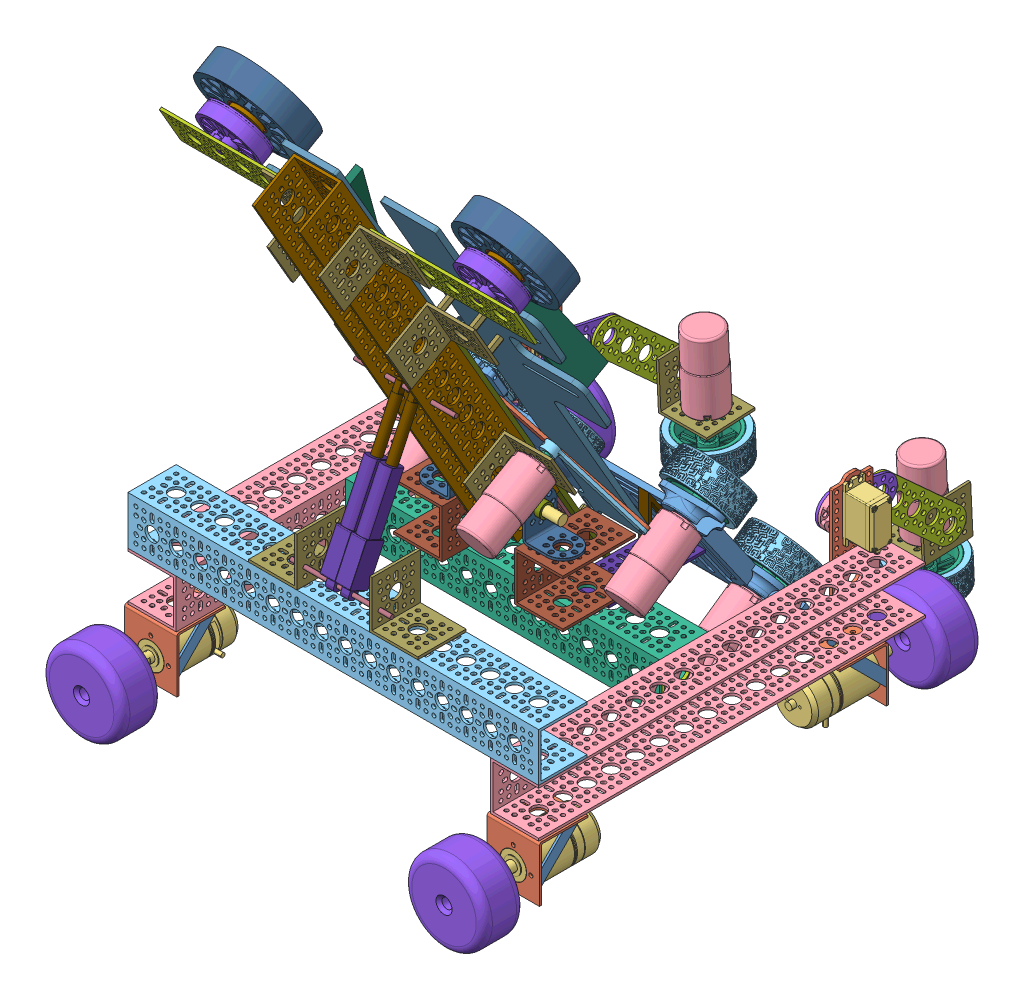
SolidWorks assembly 底座3.0, configuration 默认. Lengths in mm.
Overall size (455.34 576.17 585.99).
140 component instances, 44 part files, 283 mates.
Components (placement in the parent):
- 电机连接支架-5: 电机连接支架 [默认] at (-222.052 128.3372 691.3695) x (0 0 1) z (-1 0 0) size (48 54.5 52)
  - 小兔电机连接支架02-1: 小兔电机连接支架02 [默认] at (-18.8303 11.0829 24.6066) size (36.21 36.21 2)
  - 小兔电机连接支架02-2: 小兔电机连接支架02 [默认] at (-18.8303 11.0829 -25.3934) size (36.21 36.21 2)
  - 小兔电机连接支架-1: 小兔电机连接支架 [默认] at (17.3829 -18.9171 0.6066) size (48 54.5 52)
- 电机连接支架-6: 电机连接支架 [默认] at (137.948 128.3372 691.3695) x (0 0 1) z (-1 0 0) size (48 54.5 52)
  - 小兔电机连接支架02-1: 小兔电机连接支架02 [默认] at (-18.8303 11.0829 24.6066) size (36.21 36.21 2)
  - 小兔电机连接支架02-2: 小兔电机连接支架02 [默认] at (-18.8303 11.0829 -25.3934) size (36.21 36.21 2)
  - 小兔电机连接支架-1: 小兔电机连接支架 [默认] at (17.3829 -18.9171 0.6066) size (48 54.5 52)
- 3508无刷电机带减速箱（00）-5: 3508无刷电机带减速箱（00） [默认] at (137.3414 109.4201 681.1524) x (-1 0 0) z (0 -1 0) size (42 98.3 47)
- 3508无刷电机带减速箱（00）-7: 3508无刷电机带减速箱（00） [默认] at (-222.6586 109.4201 681.1524) x (0 -1 0) z (1 0 0) size (42 98.3 47)
- 384mm-U型梁-1: 384mm-U型梁 [默认] at (-201.1586 165.4201 709.5024) x (0 -1 0) z (1 0 0) size (48 384 48)
- 384mm-U型梁-2: 384mm-U型梁 [默认] at (115.8414 165.4201 709.5024) x (0 1 0) z (-1 0 0) size (48 384 48)
- 408mm-U型梁-10: 408mm-U型梁 [默认] at (161.3414 213.4201 707.0024) x (0 1 0) z (0 0 1) size (48 408 48)
- 312mm-U型梁-2: 312mm-U型梁 [默认] at (113.3414 165.4201 539.0024) x (0 1 0) z (0 0 1) size (48 312 48)
- 电机转向座-7: 电机转向座 [默认] at (113.3414 165.4201 517.5024) x (0 0 -1) z (0 1 0) size (43.24 12.23 43.24)
- 电机转向座-8: 电机转向座 [默认] at (-198.6586 165.4201 517.5024) x (0 0 1) z (0 1 0) size (43.24 12.23 43.24)
- 电机连接支架-7: 电机连接支架 [默认] at (136.7348 128.3372 383.6353) x (0 0 -1) z (1 0 0) size (48 54.5 52)
  - 小兔电机连接支架02-1: 小兔电机连接支架02 [默认] at (-18.8303 11.0829 24.6066) size (36.21 36.21 2)
  - 小兔电机连接支架02-2: 小兔电机连接支架02 [默认] at (-18.8303 11.0829 -25.3934) size (36.21 36.21 2)
  - 小兔电机连接支架-1: 小兔电机连接支架 [默认] at (17.3829 -18.9171 0.6066) size (48 54.5 52)
- 3508无刷电机带减速箱（00）-8: 3508无刷电机带减速箱（00） [默认] at (137.3414 109.4201 393.8524) x (1 0 0) z (0 -1 0) size (42 98.3 47)
- 电机连接支架-8: 电机连接支架 [默认] at (-223.2652 128.3372 383.6353) x (0 0 -1) z (1 0 0) size (48 54.5 52)
  - 小兔电机连接支架02-1: 小兔电机连接支架02 [默认] at (-18.8303 11.0829 24.6066) size (36.21 36.21 2)
  - 小兔电机连接支架02-2: 小兔电机连接支架02 [默认] at (-18.8303 11.0829 -25.3934) size (36.21 36.21 2)
  - 小兔电机连接支架-1: 小兔电机连接支架 [默认] at (17.3829 -18.9171 0.6066) size (48 54.5 52)
- 3508无刷电机带减速箱（00）-9: 3508无刷电机带减速箱（00） [默认] at (-222.6586 109.4201 393.8524) x (1 0 0) z (0 -1 0) size (42 98.3 47)
- 麦轮（临时）-1: 麦轮（临时） [默认] at (-222.6586 109.4201 324.5024) x (0 0 -1) z (0.996866 -0.079106 0) size (40 80 80)
- 麦轮（临时）-2: 麦轮（临时） [默认] at (137.3414 109.4201 324.5024) x (0 0 -1) z (0.923265 -0.384164 0) size (40 80 80)
- 麦轮（临时）-3: 麦轮（临时） [默认] at (137.3414 109.4201 779.5024) x (0 0 -1) z (0.99707 -0.076496 0) size (40 80 80)
- 麦轮（临时）-4: 麦轮（临时） [默认] at (-222.6586 109.4201 779.5024) x (0 0 -1) z (0.996866 -0.079106 0) size (40 80 80)
- 432mm-U型梁-1: 432mm-U型梁 [默认] at (-42.6586 251.3791 510.885) x (-1 0 0) z (0 0.499817 -0.866131) size (48 432 48)
- 圆角90°法兰-1: 圆角90°法兰 [默认] at (-6.6586 237.4201 541.5024) x (1 0 0) z (0 -1 0) size (40 32 40)
- 圆角90°法兰-2: 圆角90°法兰 [默认] at (-78.6586 237.4201 541.5024) x (-1 0 0) z (0 -1 0) size (40 32 40)
- 72mm-U型梁-1: 72mm-U型梁 [默认] at (-4.1586 213.4201 493.5024) x (0 -1 0) z (-1 0 0) size (48 72 48)
- 72mm-U型梁-2: 72mm-U型梁 [默认] at (-81.1586 213.4201 565.5024) x (0 -1 0) z (1 0 0) size (48 72 48)
- 48x48-L形支架-1: 48x48-L形支架 [默认] at (5.3414 538.4005 685.7527) x (-1 0 0) z (0 0.499817 -0.866131) size (48 48 48)
- 48x48-L形支架-3: 48x48-L形支架 [默认] at (-81.1586 261.4201 709.5024) x (0 -1 0) z (1 0 0) size (48 48 48)
- 48x48-L形支架-4: 48x48-L形支架 [默认] at (-4.1586 261.4201 661.5024) x (0 -1 0) z (-1 0 0) size (48 48 48)
- 升降轴-1: 升降轴 [默认] at (-92.6586 252.9349 701.0171) x (1 0 0) z (0 0.719401 -0.694595) size (100 4 4)
- 48x48-L形支架-5: 48x48-L形支架 [默认] at (-16.1586 319.783 584.4183) x (0 0.499817 -0.866131) z (-1 0 0) size (48 48 48)
- 滑轨-1: 滑轨 [默认] at (-45.1586 605.7383 712.4884) x (1 0 0) z (0 0.866131 0.499817) size (5 3.7 400)
- 滑块-1: 滑块 [默认] at (-42.6586 360.6986 564.1562) x (1 0 0) z (0 0.866131 0.499817) size (12 5 16)
- 铜套-1: 铜套 [默认] at (-68.6586 261.4201 541.5024) size (10 22 22)
- 铜套-2: 铜套 [默认] at (-8.6586 261.4201 541.5024) size (10 22 22)
- 铜套-3: 铜套 [默认] at (-16.6586 261.4201 541.5024) x (-1 0 0) z (0 -0.999442 0.033415) size (10 22 22)
- 铜套-4: 铜套 [默认] at (-76.6586 261.4201 541.5024) x (-1 0 0) z (0 -0.924225 -0.381849) size (10 22 22)
- 电动推杆01-1: 电动推杆01 [默认] at (-54.1586 252.9349 701.0171) x (1 0 0) z (0 -0.904213 0.427082) size (15 20 103)
- 电动推杆01-2: 电动推杆01 [默认] at (-39.1586 252.9349 701.0171) x (1 0 0) z (0 -0.904213 0.427082) size (15 20 103)
- 电动推杆2-1: 电动推杆2 [默认] at (-35.1586 336.3949 661.5968) x (-1 0 0) z (0 -0.427082 -0.904213) size (9 66 9)
- 电动推杆2-2: 电动推杆2 [默认] at (-50.1586 336.3949 661.5968) x (-1 0 0) z (0 -0.427082 -0.904213) size (9 66 9)
- 升降轴-2: 升降轴 [默认] at (-94.6586 392.004 635.3313) x (1 0 0) z (0 -0.677442 -0.735576) size (100 4 4)
- 滑块01-1: 滑块01 [默认] at (-17.6586 385.8164 578.6509) x (-1 0 0) z (0 -0.866131 -0.499817) size (50 11 45)
- 连杆02-1: 连杆02 [默认] at (-42.6586 351.771 557.6188) x (0.667921 -0.644602 -0.37198) z (0.744232 0.578507 0.333839) size (158 2.9 8)
- 10mm轴-1: 10mm轴 [默认] at (-102.6586 261.4201 541.5024) x (1 0 0) z (0 0.050897 0.998704) size (120 10 10)
- 一级摩擦轮电机01-4: 一级摩擦轮电机01 [默认] at (5.3414 273.1053 617.2883) x (-0.035714 -0.865578 -0.499499) z (0.999362 -0.030933 -0.017851) size (36 73.3 36)
- 连杆01-5: 连杆01 [默认] at (5.3414 318.5887 538.4704) x (0.579868 -0.705646 -0.407206) z (-0.81471 -0.502242 -0.289828) size (101 8 14)
- 一级摩擦轮电机02-3: 一级摩擦轮电机02 [默认] at (5.3414 308.2425 556.3993) x (-0.579868 0.705646 0.407206) z (-0.81471 -0.502242 -0.289828) size (8 20 8)
- 5孔平板-1: 5孔平板 [默认] at (133.3414 591.0546 685.5419) x (0 0.499817 -0.866131) z (0 0.866131 0.499817) size (2.5 144 43)
- 发射无刷电机-1: 发射无刷电机 [默认] at (85.3414 561.6867 693.4176) x (-0.99795 0.055432 0.031988) z (-0.064 -0.864355 -0.498793) size (58.5 35.4 58.5)
- 发射法兰-1: 发射法兰 [默认] at (85.3414 575.5816 669.3392) x (0.99795 -0.055432 -0.031988) z (0.064 0.864355 0.498793) size (30 11 30)
- 摩擦轮-2: 摩擦轮 [默认] at (91.2311 598.1447 657.2376) x (0.99795 -0.055432 -0.031988) z (0 0.499817 -0.866131) size (96 96 24)
  - 摩擦轮.STEP-1: 摩擦轮.STEP [默认] at origin size (96 96 24)
    - 3613-0014-0096 Rubber.STEP-1: 3613-0014-0096 Rubber.STEP [默认] at (-5.0141 13.8433 -6.759) size (96 96 24)
    - 3613-0014-0096 Core.STEP-1: 3613-0014-0096 Core.STEP [默认] at (-5.0141 13.8433 -6.759) x (1 0 0) z (0 -1 0) size (35.2 24 35.2)
- 摩擦轮-3: 摩擦轮 [默认] at (-176.5484 574.7696 643.7485) x (-0.99795 0.055432 0.031988) z (0 0.499817 -0.866131) size (96 96 24)
  - 摩擦轮.STEP-1: 摩擦轮.STEP [默认] at origin size (96 96 24)
    - 3613-0014-0096 Rubber.STEP-1: 3613-0014-0096 Rubber.STEP [默认] at (-5.0141 13.8433 -6.759) size (96 96 24)
    - 3613-0014-0096 Core.STEP-1: 3613-0014-0096 Core.STEP [默认] at (-5.0141 13.8433 -6.759) x (1 0 0) z (0 -1 0) size (35.2 24 35.2)
- 发射法兰-2: 发射法兰 [默认] at (-170.6586 575.5816 669.3392) x (-0.99795 0.055432 0.031988) z (-0.064 -0.864355 -0.498793) size (30 11 30)
- 发射无刷电机-3: 发射无刷电机 [默认] at (-170.6586 561.6867 693.4176) x (0.99795 -0.055432 -0.031988) z (0.064 0.864355 0.498793) size (58.5 35.4 58.5)
- 5孔平板-3: 5孔平板 [默认] at (-218.6586 553.811 664.0498) x (0 0.499817 -0.866131) z (0 -0.866131 -0.499817) size (2.5 144 43)
- 48x48-L形支架-13: 48x48-L形支架 [默认] at (-90.6586 579.9748 709.7439) x (1 0 0) z (0 0.499817 -0.866131) size (48 48 48)
- 48x48-L形支架-14: 48x48-L形支架 [默认] at (5.3414 438.4633 618.8455) x (-1 0 0) z (0 0.499817 -0.866131) size (48 48 48)
- 48x48-L形支架-15: 48x48-L形支架 [默认] at (-90.6586 480.0376 642.8368) x (1 0 0) z (0 0.499817 -0.866131) size (48 48 48)
- 铜柱-1: 铜柱 [默认] at (21.3414 474.3581 636.6729) x (1 0 0) z (0 0.866131 0.499817) size (6.93 15 6)
- 铜柱-2: 铜柱 [默认] at (21.3414 446.6419 620.6788) x (1 0 0) z (0 0.866131 0.499817) size (6.93 15 6)
- 铜柱-3: 铜柱 [默认] at (-10.6586 474.3581 636.6729) x (1 0 0) z (0 0.866131 0.499817) size (6.93 15 6)
- 铜柱-4: 铜柱 [默认] at (-74.6586 474.3581 636.6729) x (1 0 0) z (0 0.866131 0.499817) size (6.93 15 6)
- 铜柱-5: 铜柱 [默认] at (-106.6586 474.3581 636.6729) x (1 0 0) z (0 0.866131 0.499817) size (6.93 15 6)
- 铜柱-6: 铜柱 [默认] at (-106.6586 446.6419 620.6788) x (0.926042 0.326896 0.188641) z (-0.377421 0.802073 0.462852) size (6.93 15 6)
- 2孔平板-6: 2孔平板 [默认] at (-64.1586 190.8801 503.6823) x (0 -0.499817 0.866131) z (-1 0 0) size (2.5 72 43)
- 铜柱-7: 铜柱 [默认] at (-26.6586 209.8048 486.8937) x (0.868608 0.429167 0.247659) z (-0.495499 0.752328 0.434146) size (6.93 15 6)
- 铜柱-8: 铜柱 [默认] at (-58.6586 209.8048 486.8937) x (1 0 0) z (0 0.866131 0.499817) size (6.93 15 6)
- 小兔侧板-1: 小兔侧板 [默认] at (-20.6586 476.6586 620.682) x (0 -0.866131 -0.499817) z (1 0 0) size (440 5 125)
- 小兔侧板-2: 小兔侧板 [默认] at (-64.6586 479.1577 616.3514) x (0 -0.866131 -0.499817) z (-1 0 0) size (440 5 125)
- 滚针版-1: 滚针版 [默认] at (74.3414 416.6254 580.2659) x (0 0.499817 -0.866131) z (-0.341232 0.814145 0.469818) size (31 6 130)
- 滚针版-2: 滚针版 [默认] at (-154.0188 414.8521 579.2426) x (0 0.499817 -0.866131) z (0.341232 0.814145 0.469818) size (31 6 130)
- 抓钩滑轨-1: 抓钩滑轨 [默认] at (-19.1586 429.5863 606.2182) x (0 -0.866131 -0.499817) z (1 0 0) size (300 4 15)
- 抓钩滑轨-2: 抓钩滑轨 [默认] at (-51.1586 429.5863 606.2182) x (0 -0.866131 -0.499817) z (1 0 0) size (300 4 15)
- 3孔平板-1: 3孔平板 [默认] at (38.8414 208.4201 421.5024) x (0 1 0) z (1 0 0) size (2.5 96 43)
- 03铲板支架-1: 03铲板支架 [默认] at (6.3414 186.9201 445.5024) size (10 45 28.75)
- 铲板-1: 铲板 [默认] at (-137.6586 235.5843 441.9642) x (1 0 0) z (0 0.819152 0.573576) size (290 21.92 257.38)
- 舵机支架-1: 舵机支架 [默认] at (113.3414 223.4201 349.5024) x (0 1 0) z (0 0 1) size (109.25 3.14 40)
- 舵机-1: 舵机 [默认] at (104.8414 223.4201 349.4524) x (0 1 0) z (-1 0 0) size (54.3 20 43.9)
- 舵机支架-2: 舵机支架 [默认] at (-198.6586 223.4201 349.5024) x (0 1 0) z (0 0 -1) size (109.25 3.14 40)
- 舵机-2: 舵机 [默认] at (-190.1586 223.4201 349.5524) x (0 1 0) z (1 0 0) size (54.3 20 43.9)
- 舵机法兰-1: 舵机法兰 [默认] at (102.5414 213.5701 349.4524) x (0 0.835132 0.55005) z (0 -0.55005 0.835132) size (31.98 8.12 31.98)
- 舵机法兰-2: 舵机法兰 [默认] at (-187.8586 213.5701 349.5524) x (0 -0.547519 0.836794) z (0 0.836794 0.547519) size (31.98 8.12 31.98)
- 一级摩擦轮电机01-6: 一级摩擦轮电机01 [默认] at (-150.8586 190.9516 233.9904) x (-0.999362 -0.001717 0.035673) z (0.035714 -0.048045 0.998206) size (36 73.3 36)
- 一级摩擦轮电机02-5: 一级摩擦轮电机02 [默认] at (-150.8586 120.7329 230.6107) x (-0.010219 0.048073 -0.998792) z (-0.999948 -0.000491 0.010207) size (8 20 8)
- 蓝色橡胶轮胎-1: 蓝色橡胶轮胎 [默认] at (-115.6643 102.8382 197.3636) x (-0.999113 0.002024 -0.042051) z (0 0.998844 0.048076) size (67.13 67.1 31.57)
  - 蓝色橡胶轮胎.stp-1: 蓝色橡胶轮胎.stp [默认] at origin size (67.13 67.1 31.57)
    - PRT0002.stp-1: PRT0002.stp [默认] at (33.8013 60.8485 -25.75) size (67.13 67.1 26.5)
    - LUNGU2.stp-1: LUNGU2.stp [默认] at (61.1013 33.7786 -26.4276) x (0 0 1) z (-1 0.000833 0) size (31.5 54.6 54.6)
- 圆角孔板5孔-2: 圆角孔板5孔 [默认] at (-177.3586 203.7518 302.5673) x (0 -0.672295 -0.740284) z (0 -0.740284 0.672295) size (128 2.5 32)
- 48x48-L形支架-16: 48x48-L形支架 [默认] at (-172.3586 140.3654 207.5278) x (0 -0.998844 -0.048076) z (-1 0 0) size (48 48 48)
- 圆角孔板3孔-2: 圆角孔板3孔 [默认] at (-177.3586 213.5701 349.5524) x (0 -0.204548 -0.978856) z (0 0.978856 -0.204548) size (80 2.5 32)
- 圆角孔板3孔-3: 圆角孔板3孔 [默认] at (94.5414 213.5701 349.4524) x (0 -0.201583 -0.979471) z (0 0.979471 -0.201583) size (80 2.5 32)
- 圆角孔板5孔-3: 圆角孔板5孔 [默认] at (89.5414 203.8941 302.4378) x (0 -0.673777 -0.738935) z (0 -0.738935 0.673777) size (128 2.5 32)
- 48x48-L形支架-17: 48x48-L形支架 [默认] at (87.0414 138.0577 255.4723) x (0 -0.998844 -0.048076) z (1 0 0) size (48 48 48)
- 一级摩擦轮电机02-6: 一级摩擦轮电机02 [默认] at (65.5414 120.7329 230.6107) x (-0.010158 0.048073 -0.998792) z (-0.999948 -0.000488 0.010147) size (8 20 8)
- 一级摩擦轮电机01-7: 一级摩擦轮电机01 [默认] at (65.5414 190.9516 233.9904) x (0.999362 0.001717 -0.035673) z (-0.035714 0.048045 -0.998206) size (36 73.3 36)
- 蓝色橡胶轮胎-2: 蓝色橡胶轮胎 [默认] at (100.713 102.8394 197.3389) x (-0.999143 0.00199 -0.04135) z (0 0.998844 0.048076) size (67.13 67.1 31.57)
  - 蓝色橡胶轮胎.stp-1: 蓝色橡胶轮胎.stp [默认] at origin size (67.13 67.1 31.57)
    - PRT0002.stp-1: PRT0002.stp [默认] at (33.8013 60.8485 -25.75) size (67.13 67.1 26.5)
    - LUNGU2.stp-1: LUNGU2.stp [默认] at (61.1013 33.7786 -26.4276) x (0 0 1) z (-1 0.000833 0) size (31.5 54.6 54.6)
- 一级摩擦轮电机01-8: 一级摩擦轮电机01 [默认] at (-152.6586 111.2138 462.6735) x (-1 0 0) z (0 -0.819152 -0.573576) size (36 73.3 36)
- 一级摩擦轮电机02-7: 一级摩擦轮电机02 [默认] at (-152.6586 151.5363 405.0871) x (0.972137 -0.192019 -0.134453) z (0.234412 0.796328 0.557595) size (8 20 8)
- 蓝色橡胶轮胎-3: 蓝色橡胶轮胎 [默认] at (-139.2945 200.3011 415.4612) x (-0.876598 -0.394195 -0.276018) z (0 -0.573576 0.819152) size (67.13 67.1 31.57)
  - 蓝色橡胶轮胎.stp-1: 蓝色橡胶轮胎.stp [默认] at origin size (67.13 67.1 31.57)
    - PRT0002.stp-1: PRT0002.stp [默认] at (33.8013 60.8485 -25.75) size (67.13 67.1 26.5)
    - LUNGU2.stp-1: LUNGU2.stp [默认] at (61.1013 33.7786 -26.4276) x (0 0 1) z (-1 0.000833 0) size (31.5 54.6 54.6)
- 一级摩擦轮电机01-9: 一级摩擦轮电机01 [默认] at (67.3414 111.2138 462.6735) x (-1 0 0) z (0 -0.819152 -0.573576) size (36 73.3 36)
- 一级摩擦轮电机01-10: 一级摩擦轮电机01 [默认] at (67.3414 209.5121 531.5026) x (-1 0 0) z (0 -0.819152 -0.573576) size (36 73.3 36)
- 一级摩擦轮电机01-11: 一级摩擦轮电机01 [默认] at (-152.6586 209.5121 531.5026) x (-1 0 0) z (0 -0.819152 -0.573576) size (36 73.3 36)
- 蓝色橡胶轮胎-4: 蓝色橡胶轮胎 [默认] at (-173.4894 225.7595 433.2874) x (0.944573 0.268929 0.188306) z (0 -0.573576 0.819152) size (67.13 67.1 31.57)
  - 蓝色橡胶轮胎.stp-1: 蓝色橡胶轮胎.stp [默认] at origin size (67.13 67.1 31.57)
    - PRT0002.stp-1: PRT0002.stp [默认] at (33.8013 60.8485 -25.75) size (67.13 67.1 26.5)
    - LUNGU2.stp-1: LUNGU2.stp [默认] at (61.1013 33.7786 -26.4276) x (0 0 1) z (-1 0.000833 0) size (31.5 54.6 54.6)
- 蓝色橡胶轮胎-5: 蓝色橡胶轮胎 [默认] at (26.3553 142.5534 375.0258) x (0.970182 -0.198543 -0.139022) z (0 -0.573576 0.819152) size (67.13 67.1 31.57)
  - 蓝色橡胶轮胎.stp-1: 蓝色橡胶轮胎.stp [默认] at origin size (67.13 67.1 31.57)
    - PRT0002.stp-1: PRT0002.stp [默认] at (33.8013 60.8485 -25.75) size (67.13 67.1 26.5)
    - LUNGU2.stp-1: LUNGU2.stp [默认] at (61.1013 33.7786 -26.4276) x (0 0 1) z (-1 0.000833 0) size (31.5 54.6 54.6)
- 蓝色橡胶轮胎-6: 蓝色橡胶轮胎 [默认] at (23.7949 244.8521 446.6561) x (0.935815 -0.288744 -0.202181) z (0 -0.573576 0.819152) size (67.13 67.1 31.57)
  - 蓝色橡胶轮胎.stp-1: 蓝色橡胶轮胎.stp [默认] at origin size (67.13 67.1 31.57)
    - PRT0002.stp-1: PRT0002.stp [默认] at (33.8013 60.8485 -25.75) size (67.13 67.1 26.5)
    - LUNGU2.stp-1: LUNGU2.stp [默认] at (61.1013 33.7786 -26.4276) x (0 0 1) z (-1 0.000833 0) size (31.5 54.6 54.6)
- 一级摩擦轮电机02-8: 一级摩擦轮电机02 [默认] at (-152.6586 249.8345 473.9162) x (0.616796 -0.644774 -0.451475) z (0.787123 0.50525 0.35378) size (8 20 8)
- 一级摩擦轮电机02-9: 一级摩擦轮电机02 [默认] at (67.3414 249.8345 473.9162) x (0.616796 -0.644774 -0.451475) z (0.787123 0.50525 0.35378) size (8 20 8)
- 一级摩擦轮电机02-10: 一级摩擦轮电机02 [默认] at (67.3414 151.5363 405.0871) x (0.616796 -0.644774 -0.451475) z (0.787123 0.50525 0.35378) size (8 20 8)
Mates (geometry in assembly coordinates):
- Coincident37: coincident anti-aligned: plane of 电机连接支架-5/小兔电机连接支架-1 through (-222.6586 109.4201 708.7524) normal (0 0 -1); plane of 3508无刷电机带减速箱（00）-7 through (-222.6586 96.4201 708.7524) normal (0 0 1)
- Concentric38: concentric aligned: cylinder of 电机连接支架-5/小兔电机连接支架-1 through (-222.6586 109.4201 710.7524) axis (0 0 -1) radius 13.25; cylinder of 3508无刷电机带减速箱（00）-7 through (-222.6586 109.4201 672.4524) axis (0 0 -1) radius 13
- Concentric39: concentric anti-aligned: cylinder of 电机连接支架-5/小兔电机连接支架-1 through (-222.6586 126.9201 710.7524) axis (0 0 -1) radius 2; cylinder of 3508无刷电机带减速箱（00）-7 through (-222.6586 126.9201 708.7524) axis (0 0 1) radius 1.65
- Coincident38: coincident anti-aligned: plane of 电机连接支架-6/小兔电机连接支架-1 through (137.3414 109.4201 708.7524) normal (0 0 -1); plane of 3508无刷电机带减速箱（00）-5 through (124.3414 109.4201 708.7524) normal (0 0 1)
- Concentric40: concentric aligned: cylinder of 电机连接支架-6/小兔电机连接支架-1 through (137.3414 109.4201 710.7524) axis (0 0 -1) radius 13.25; cylinder of 3508无刷电机带减速箱（00）-5 through (137.3414 109.4201 672.4524) axis (0 0 -1) radius 13
- Concentric41: concentric anti-aligned: cylinder of 电机连接支架-6/小兔电机连接支架-1 through (137.3414 126.9201 710.7524) axis (0 0 -1) radius 2; cylinder of 3508无刷电机带减速箱（00）-5 through (137.3414 126.9201 708.7524) axis (0 0 1) radius 1.65
- Concentric261: concentric anti-aligned: cylinder of 384mm-U型梁-2 through (137.3414 179.4201 685.5024) axis (0 1 0) radius 7; cylinder of 408mm-U型梁-10 through (137.3414 199.4201 685.5024) axis (0 -1 0) radius 7
- Concentric262: concentric anti-aligned: cylinder of 384mm-U型梁-1 through (-222.6586 179.4201 685.5024) axis (0 1 0) radius 7; cylinder of 408mm-U型梁-10 through (-222.6586 199.4201 685.5024) axis (0 -1 0) radius 7
- Coincident94: coincident aligned: plane of 384mm-U型梁-2 through (161.3414 186.9201 325.5024) normal (1 0 0); plane of 408mm-U型梁-10 through (161.3414 213.4201 707.0024) normal (1 0 0)
- Coincident95: coincident aligned: plane of 384mm-U型梁-1 through (-246.6586 186.9201 325.5024) normal (-1 0 0); plane of 408mm-U型梁-10 through (-246.6586 213.4201 707.0024) normal (-1 0 0)
- Coincident96: coincident anti-aligned: plane of 384mm-U型梁-1 through (-246.6586 189.4201 325.5024) normal (0 1 0); plane of 408mm-U型梁-10 through (-246.6586 189.4201 661.5024) normal (0 -1 0)
- Coincident97: coincident anti-aligned: plane of 384mm-U型梁-2 through (161.3414 189.4201 325.5024) normal (0 1 0); plane of 408mm-U型梁-10 through (-246.6586 189.4201 661.5024) normal (0 -1 0)
- Concentric267: concentric aligned: cylinder of 电机连接支架-7/小兔电机连接支架-1 through (137.3414 109.4201 364.2524) axis (0 0 1) radius 13.25; cylinder of 3508无刷电机带减速箱（00）-8 through (137.3414 109.4201 402.5524) axis (0 0 1) radius 13
- Coincident104: coincident anti-aligned: plane of 电机连接支架-7/小兔电机连接支架-1 through (137.3414 109.4201 366.2524) normal (0 0 1); plane of 3508无刷电机带减速箱（00）-8 through (150.3414 109.4201 366.2524) normal (0 0 -1)
- Concentric268: concentric anti-aligned: cylinder of 电机连接支架-7/小兔电机连接支架-1 through (137.3414 126.9201 364.2524) axis (0 0 1) radius 2; cylinder of 3508无刷电机带减速箱（00）-8 through (137.3414 126.9201 366.2524) axis (0 0 -1) radius 1.65
- Concentric269: concentric aligned: cylinder of 电机连接支架-8/小兔电机连接支架-1 through (-222.6586 109.4201 364.2524) axis (0 0 1) radius 13.25; cylinder of 3508无刷电机带减速箱（00）-9 through (-222.6586 109.4201 402.5524) axis (0 0 1) radius 13
- Coincident105: coincident anti-aligned: plane of 电机连接支架-8/小兔电机连接支架-1 through (-222.6586 109.4201 366.2524) normal (0 0 1); plane of 3508无刷电机带减速箱（00）-9 through (-209.6586 109.4201 366.2524) normal (0 0 -1)
- Concentric270: concentric anti-aligned: cylinder of 电机连接支架-8/小兔电机连接支架-1 through (-222.6586 126.9201 364.2524) axis (0 0 1) radius 2; cylinder of 3508无刷电机带减速箱（00）-9 through (-222.6586 126.9201 366.2524) axis (0 0 -1) radius 1.65
- Concentric271: concentric anti-aligned: cylinder of 电机连接支架-6/小兔电机连接支架-1 through (137.3414 86.9201 685.5024) axis (0 1 0) radius 7; cylinder of 384mm-U型梁-2 through (137.3414 151.4201 685.5024) axis (0 -1 0) radius 7
- Coincident106: coincident anti-aligned: plane of 电机连接支架-6/小兔电机连接支架-1 through (163.3414 141.4201 662.7524) normal (0 1 0); plane of 384mm-U型梁-2 through (161.3414 141.4201 325.5024) normal (0 -1 0)
- Concentric272: concentric anti-aligned: cylinder of 电机连接支架-6/小兔电机连接支架-1 through (153.3414 86.9201 701.5024) axis (0 1 0) radius 2; cylinder of 384mm-U型梁-2 through (153.3414 151.4201 701.5024) axis (0 -1 0) radius 2
- Concentric273: concentric anti-aligned: cylinder of 电机连接支架-5/小兔电机连接支架-1 through (-222.6586 86.9201 685.5024) axis (0 1 0) radius 7; cylinder of 384mm-U型梁-1 through (-222.6586 151.4201 685.5024) axis (0 -1 0) radius 7
- Coincident107: coincident anti-aligned: plane of 电机连接支架-5/小兔电机连接支架-1 through (-196.6586 141.4201 662.7524) normal (0 1 0); plane of 384mm-U型梁-1 through (-246.6586 141.4201 325.5024) normal (0 -1 0)
- Concentric274: concentric anti-aligned: cylinder of 电机连接支架-5/小兔电机连接支架-1 through (-206.6586 86.9201 701.5024) axis (0 1 0) radius 2; cylinder of 384mm-U型梁-1 through (-206.6586 151.4201 701.5024) axis (0 -1 0) radius 2
- Coincident108: coincident anti-aligned: plane of 384mm-U型梁-2 through (161.3414 141.4201 325.5024) normal (0 -1 0); plane of 电机连接支架-7/小兔电机连接支架-1 through (111.3414 141.4201 412.2524) normal (0 1 0)
- Concentric276: concentric anti-aligned: cylinder of 384mm-U型梁-2 through (153.3414 151.4201 373.5024) axis (0 -1 0) radius 2; cylinder of 电机连接支架-7/小兔电机连接支架-1 through (153.3414 86.9201 373.5024) axis (0 1 0) radius 2
- Concentric277: concentric anti-aligned: cylinder of 384mm-U型梁-2 through (121.3414 151.4201 373.5024) axis (0 -1 0) radius 2; cylinder of 电机连接支架-7/小兔电机连接支架-1 through (121.3414 86.9201 373.5024) axis (0 1 0) radius 2
- Coincident109: coincident anti-aligned: plane of 384mm-U型梁-1 through (-246.6586 141.4201 325.5024) normal (0 -1 0); plane of 电机连接支架-8/小兔电机连接支架-1 through (-248.6586 141.4201 412.2524) normal (0 1 0)
- Concentric278: concentric anti-aligned: cylinder of 384mm-U型梁-1 through (-238.6586 151.4201 373.5024) axis (0 -1 0) radius 2; cylinder of 电机连接支架-8/小兔电机连接支架-1 through (-238.6586 86.9201 373.5024) axis (0 1 0) radius 2
- Concentric279: concentric anti-aligned: cylinder of 384mm-U型梁-1 through (-206.6586 151.4201 373.5024) axis (0 -1 0) radius 2; cylinder of 电机连接支架-8/小兔电机连接支架-1 through (-206.6586 86.9201 373.5024) axis (0 1 0) radius 2
- Concentric280: concentric anti-aligned: cylinder of 3508无刷电机带减速箱（00）-9 through (-222.6586 109.4201 402.5524) axis (0 0 1) radius 5; cylinder of 麦轮（临时）-1 through (-222.6586 109.4201 324.5024) axis (0 0 -1) radius 5
- Distance1: distance = 1 mm anti-aligned: plane of 麦轮（临时）-1 through (-222.6586 109.4201 324.5024) normal (0 0 1); plane of 384mm-U型梁-1 through (-201.1586 165.4201 325.5024) normal (0 0 -1)
- Concentric281: concentric anti-aligned: cylinder of 3508无刷电机带减速箱（00）-8 through (137.3414 109.4201 402.5524) axis (0 0 1) radius 5; cylinder of 麦轮（临时）-2 through (137.3414 109.4201 324.5024) axis (0 0 -1) radius 5
- Distance2: distance = 1 mm anti-aligned: plane of 384mm-U型梁-2 through (115.8414 165.4201 325.5024) normal (0 0 -1); plane of 麦轮（临时）-2 through (137.3414 109.4201 324.5024) normal (0 0 1)
- Concentric282: concentric aligned: cylinder of 3508无刷电机带减速箱（00）-5 through (137.3414 109.4201 672.4524) axis (0 0 -1) radius 5; cylinder of 麦轮（临时）-3 through (137.3414 109.4201 779.5024) axis (0 0 -1) radius 5
- Distance3: distance = 495 mm anti-aligned: plane of 麦轮（临时）-3 through (137.3414 109.4201 779.5024) normal (0 0 1); plane of 麦轮（临时）-2 through (137.3414 109.4201 284.5024) normal (0 0 -1)
- Concentric283: concentric aligned: cylinder of 3508无刷电机带减速箱（00）-7 through (-222.6586 109.4201 672.4524) axis (0 0 -1) radius 5; cylinder of 麦轮（临时）-4 through (-222.6586 109.4201 779.5024) axis (0 0 -1) radius 5
- Distance4: distance = 495 mm anti-aligned: plane of 麦轮（临时）-4 through (-222.6586 109.4201 779.5024) normal (0 0 1); plane of 麦轮（临时）-1 through (-222.6586 109.4201 284.5024) normal (0 0 -1)
- Concentric290: concentric anti-aligned: cylinder of 312mm-U型梁-2 through (17.3414 179.4201 517.5024) axis (0 1 0) radius 7; cylinder of 72mm-U型梁-1 through (17.3414 199.4201 517.5024) axis (0 -1 0) radius 7
- Concentric291: concentric anti-aligned: cylinder of 312mm-U型梁-2 through (1.3414 179.4201 501.5024) axis (0 1 0) radius 2; cylinder of 72mm-U型梁-1 through (1.3414 199.4201 501.5024) axis (0 -1 0) radius 2
- Coincident112: coincident anti-aligned: plane of 312mm-U型梁-2 through (-198.6586 189.4201 493.5024) normal (0 1 0); plane of 72mm-U型梁-1 through (41.3414 189.4201 565.5024) normal (0 -1 0)
- Concentric292: concentric aligned: cylinder of 圆角90°法兰-1 through (17.3414 237.4201 541.5024) axis (0 1 0) radius 7; cylinder of 72mm-U型梁-1 through (17.3414 227.4201 541.5024) axis (0 1 0) radius 7
- Coincident113: coincident anti-aligned: plane of 圆角90°法兰-1 through (-6.6586 237.4201 557.5024) normal (0 -1 0); plane of 72mm-U型梁-1 through (41.3414 237.4201 565.5024) normal (0 1 0)
- Concentric293: concentric aligned: cylinder of 圆角90°法兰-1 through (9.3414 237.4201 533.5024) axis (0 1 0) radius 2.025; cylinder of 72mm-U型梁-1 through (9.3414 227.4201 533.5024) axis (0 1 0) radius 2
- Concentric294: concentric anti-aligned: cylinder of 312mm-U型梁-2 through (-102.6586 179.4201 517.5024) axis (0 1 0) radius 7; cylinder of 72mm-U型梁-2 through (-102.6586 199.4201 517.5024) axis (0 -1 0) radius 7
- Coincident114: coincident anti-aligned: plane of 312mm-U型梁-2 through (-198.6586 189.4201 493.5024) normal (0 1 0); plane of 72mm-U型梁-2 through (-126.6586 189.4201 493.5024) normal (0 -1 0)
- Concentric295: concentric anti-aligned: cylinder of 312mm-U型梁-2 through (-86.6586 179.4201 501.5024) axis (0 1 0) radius 2; cylinder of 72mm-U型梁-2 through (-86.6586 199.4201 501.5024) axis (0 -1 0) radius 2
- Concentric296: concentric aligned: cylinder of 圆角90°法兰-2 through (-102.6586 237.4201 541.5024) axis (0 1 0) radius 7; cylinder of 72mm-U型梁-2 through (-102.6586 227.4201 541.5024) axis (0 1 0) radius 7
- Coincident115: coincident anti-aligned: plane of 圆角90°法兰-2 through (-78.6586 237.4201 525.5024) normal (0 -1 0); plane of 72mm-U型梁-2 through (-126.6586 237.4201 493.5024) normal (0 1 0)
- Concentric297: concentric aligned: cylinder of 圆角90°法兰-2 through (-110.6586 237.4201 549.5024) axis (0 1 0) radius 2.025; cylinder of 72mm-U型梁-2 through (-110.6586 227.4201 549.5024) axis (0 1 0) radius 2
- Concentric298: concentric aligned: cylinder of 432mm-U型梁-1 through (-28.6586 261.4201 541.5024) axis (1 0 0) radius 7; cylinder of 圆角90°法兰-1 through (-6.6586 261.4201 541.5024) axis (1 0 0) radius 7
- Distance5: distance = 12 mm anti-aligned: plane of 432mm-U型梁-1 through (-18.6586 602.8059 766.2151) normal (1 0 0); plane of 圆角90°法兰-1 through (-6.6586 237.4201 557.5024) normal (-1 0 0)
- Coincident120: coincident anti-aligned: plane of 408mm-U型梁-10 through (-246.6586 237.4201 661.5024) normal (0 1 0); plane of 48x48-L形支架-3 through (-126.6586 237.4201 661.5024) normal (0 -1 0)
- Concentric309: concentric anti-aligned: cylinder of 408mm-U型梁-10 through (-102.6586 227.4201 685.5024) axis (0 1 0) radius 7; cylinder of 48x48-L形支架-3 through (-102.6586 247.4201 685.5024) axis (0 -1 0) radius 7
- Concentric310: concentric anti-aligned: cylinder of 408mm-U型梁-10 through (-118.6586 227.4201 669.5024) axis (0 1 0) radius 2; cylinder of 48x48-L形支架-3 through (-118.6586 247.4201 669.5024) axis (0 -1 0) radius 2
- Concentric311: concentric anti-aligned: cylinder of 408mm-U型梁-10 through (17.3414 227.4201 685.5024) axis (0 1 0) radius 7; cylinder of 48x48-L形支架-4 through (17.3414 247.4201 685.5024) axis (0 -1 0) radius 7
- Coincident121: coincident anti-aligned: plane of 408mm-U型梁-10 through (-246.6586 237.4201 661.5024) normal (0 1 0); plane of 48x48-L形支架-4 through (41.3414 237.4201 709.5024) normal (0 -1 0)
- Concentric312: concentric anti-aligned: cylinder of 408mm-U型梁-10 through (1.3414 227.4201 701.5024) axis (0 1 0) radius 2; cylinder of 48x48-L形支架-4 through (1.3414 247.4201 701.5024) axis (0 -1 0) radius 2
- Concentric313: concentric anti-aligned: cylinder of 48x48-L形支架-3 through (-88.6586 252.9349 701.0171) axis (1 0 0) radius 2; cylinder of 升降轴-1 through (7.3414 252.9349 701.0171) axis (-1 0 0) radius 2
- Distance6: distance = 11.5 mm aligned: plane of 升降轴-1 through (-92.6586 252.9349 701.0171) normal (-1 0 0); plane of 48x48-L形支架-3 through (-81.1586 282.9201 661.5024) normal (-1 0 0)
- Coincident122: coincident anti-aligned: plane of 432mm-U型梁-1 through (-18.6586 602.8059 766.2151) normal (1 0 0); plane of 48x48-L形支架-5 through (-18.6586 290.2044 539.6399) normal (-1 0 0)
- Coincident123: coincident anti-aligned: plane of 432mm-U型梁-1 through (-66.6586 626.7971 724.6408) normal (0 0.499817 -0.866131); plane of 滑轨-1 through (-40.1586 259.2859 512.5614) normal (0 -0.499817 0.866131)
- Concentric316: concentric aligned: cylinder of 432mm-U型梁-1 through (-42.6586 258.6184 523.7218) axis (0 0.499817 -0.866131) radius 2; cylinder of 滑轨-1 through (-42.6586 263.6166 515.0605) axis (0 0.499817 -0.866131) radius 1
- Slot1: slot aligned: cylinder of 滑轨-1 through (-42.6586 575.4237 694.9948) axis (0 0.499817 -0.866131) radius 1; plane of 432mm-U型梁-1 through (-44.6586 569.8311 703.313) normal (1 0 0); cylinder of 432mm-U型梁-1 through (-42.6586 569.2367 702.97) axis (0 0.499817 -0.866131) radius 2
- Coincident124: coincident anti-aligned: plane of 滑轨-1 through (-45.1586 261.1353 509.3567) normal (0 0.499817 -0.866131); plane of 滑块-1 through (-45.1586 373.4071 574.1453) normal (0 -0.499817 0.866131)
- Coincident125: coincident anti-aligned: plane of 滑轨-1 through (-45.1586 259.2859 512.5614) normal (-1 0 0); plane of 滑块-1 through (-45.1586 372.9073 575.0115) normal (1 0 0)
- Concentric318: concentric aligned: cylinder of 432mm-U型梁-1 through (-56.6586 261.4201 541.5024) axis (-1 0 0) radius 7; cylinder of 铜套-1 through (-58.6586 261.4201 541.5024) axis (-1 0 0) radius 7
- Coincident127: coincident anti-aligned: plane of 432mm-U型梁-1 through (-66.6586 602.8059 766.2151) normal (-1 0 0); plane of 铜套-1 through (-66.6586 261.4201 541.5024) normal (1 0 0)
- Concentric319: concentric anti-aligned: cylinder of 圆角90°法兰-1 through (-6.6586 261.4201 541.5024) axis (1 0 0) radius 7; cylinder of 铜套-2 through (1.3414 261.4201 541.5024) axis (-1 0 0) radius 7
- Coincident128: coincident anti-aligned: plane of 圆角90°法兰-1 through (-6.6586 237.4201 557.5024) normal (-1 0 0); plane of 铜套-2 through (-6.6586 261.4201 541.5024) normal (1 0 0)
- Concentric320: concentric aligned: cylinder of 432mm-U型梁-1 through (-28.6586 261.4201 541.5024) axis (1 0 0) radius 7; cylinder of 铜套-3 through (-26.6586 261.4201 541.5024) axis (1 0 0) radius 7
- Coincident129: coincident anti-aligned: plane of 432mm-U型梁-1 through (-18.6586 602.8059 766.2151) normal (1 0 0); plane of 铜套-3 through (-18.6586 261.4201 541.5024) normal (-1 0 0)
- Concentric322: concentric anti-aligned: cylinder of 圆角90°法兰-2 through (-78.6586 261.4201 541.5024) axis (-1 0 0) radius 7; cylinder of 铜套-4 through (-86.6586 261.4201 541.5024) axis (1 0 0) radius 7
- Coincident130: coincident anti-aligned: plane of 圆角90°法兰-2 through (-78.6586 237.4201 525.5024) normal (1 0 0); plane of 铜套-4 through (-78.6586 261.4201 541.5024) normal (-1 0 0)
- Concentric323: concentric aligned: cylinder of 升降轴-1 through (7.3414 252.9349 701.0171) axis (-1 0 0) radius 2; cylinder of 电动推杆01-1 through (-46.1586 252.9349 701.0171) axis (-1 0 0) radius 2
- Concentric324: concentric aligned: cylinder of 升降轴-1 through (7.3414 252.9349 701.0171) axis (-1 0 0) radius 2; cylinder of 电动推杆01-2 through (-31.1586 252.9349 701.0171) axis (-1 0 0) radius 2
- Concentric325: concentric anti-aligned: cylinder of 电动推杆01-2 through (-35.1586 292.2681 682.439) axis (0 0.904213 -0.427082) radius 4.5; cylinder of 电动推杆2-1 through (-35.1586 386.1266 638.1073) axis (0 -0.904213 0.427082) radius 4.5
- LimitDistance1: limit distance = 6.1987 mm anti-aligned: plane of 电动推杆2-1 through (-35.1586 336.3949 661.5968) normal (0 -0.904213 0.427082); plane of 电动推杆01-2 through (-35.1586 341.9998 658.9495) normal (0 0.904213 -0.427082)
- LimitDistance2: limit distance = 48.8013 mm aligned: plane of 电动推杆2-1 through (-35.1586 386.1266 638.1073) normal (0 0.904213 -0.427082); plane of 电动推杆01-2 through (-35.1586 341.9998 658.9495) normal (0 0.904213 -0.427082)
- Concentric328: concentric anti-aligned: cylinder of 电动推杆01-1 through (-50.1586 292.2681 682.439) axis (0 0.904213 -0.427082) radius 4.5; cylinder of 电动推杆2-2 through (-50.1586 386.1266 638.1073) axis (0 -0.904213 0.427082) radius 4.5
- LimitDistance6: limit distance = 6.1987 mm anti-aligned: plane of 电动推杆01-1 through (-50.1586 341.9998 658.9495) normal (0 0.904213 -0.427082); plane of 电动推杆2-2 through (-50.1586 336.3949 661.5968) normal (0 -0.904213 0.427082)
- LimitDistance7: limit distance = 48.8013 mm aligned: plane of 电动推杆2-2 through (-50.1586 386.1266 638.1073) normal (0 0.904213 -0.427082); plane of 电动推杆01-1 through (-50.1586 341.9998 658.9495) normal (0 0.904213 -0.427082)
- Coincident131: coincident anti-aligned: plane of 电动推杆01-1 through (-42.6586 287.9973 673.3969) normal (1 0 0); plane of 电动推杆01-2 through (-42.6586 296.5389 691.4812) normal (-1 0 0)
- Distance12: distance = 21 mm anti-aligned: plane of 电动推杆01-1 through (-57.6586 296.5389 691.4812) normal (-1 0 0); plane of 48x48-L形支架-3 through (-78.6586 237.4201 661.5024) normal (1 0 0)
- Concentric332: concentric anti-aligned: cylinder of 432mm-U型梁-1 through (-56.6586 392.004 635.3313) axis (-1 0 0) radius 2; cylinder of 电动推杆2-2 through (-54.6586 392.004 635.3313) axis (1 0 0) radius 2
- Concentric333: concentric aligned: cylinder of 432mm-U型梁-1 through (-28.6586 392.004 635.3313) axis (1 0 0) radius 2; cylinder of 电动推杆2-1 through (-39.6586 392.004 635.3313) axis (1 0 0) radius 2
- Concentric334: concentric anti-aligned: cylinder of 432mm-U型梁-1 through (-28.6586 392.004 635.3313) axis (1 0 0) radius 2; cylinder of 升降轴-2 through (5.3414 392.004 635.3313) axis (-1 0 0) radius 2
- Coincident133: coincident anti-aligned: plane of 滑块-1 through (-36.6586 374.5567 572.1532) normal (0 0.499817 -0.866131); plane of 滑块01-1 through (-64.6586 383.218 577.1514) normal (0 -0.499817 0.866131)
- Concentric335: concentric aligned: cylinder of 滑块-1 through (-38.6586 359.6306 582.0128) axis (0 0.499817 -0.866131) radius 0.8; cylinder of 滑块01-1 through (-38.6586 367.6277 568.1547) axis (0 0.499817 -0.866131) radius 1.05
- Concentric336: concentric aligned: cylinder of 滑块-1 through (-46.6586 359.6306 582.0128) axis (0 0.499817 -0.866131) radius 0.8; cylinder of 滑块01-1 through (-46.6586 367.6277 568.1547) axis (0 0.499817 -0.866131) radius 1.05
- Concentric342: concentric aligned: cylinder of 滑块01-1 through (-42.6586 355.1697 551.7291) axis (0 -0.499817 0.866131) radius 1.6; cylinder of 连杆02-1 through (-42.6586 353.2204 555.107) axis (0 -0.499817 0.866131) radius 1.6
- Coincident137: coincident anti-aligned: plane of 滑块01-1 through (-57.6586 357.5511 557.6061) normal (0 -0.499817 0.866131); plane of 连杆02-1 through (-42.6586 353.2204 555.107) normal (0 0.499817 -0.866131)
- Concentric348: concentric anti-aligned: cylinder of 432mm-U型梁-1 through (-28.6586 320.851 566.5617) axis (1 0 0) radius 2; cylinder of 48x48-L形支架-5 through (-8.6586 320.851 566.5617) axis (-1 0 0) radius 2
- Concentric349: concentric anti-aligned: cylinder of 432mm-U型梁-1 through (-28.6586 293.1349 550.5675) axis (1 0 0) radius 2; cylinder of 48x48-L形支架-5 through (-8.6586 293.1349 550.5675) axis (-1 0 0) radius 2
- Concentric414: concentric anti-aligned: cylinder of 铜套-2 through (-8.6586 261.4201 541.5024) axis (1 0 0) radius 5; cylinder of 10mm轴-1 through (17.3414 261.4201 541.5024) axis (-1 0 0) radius 5
- Distance13: distance = 16 mm aligned: plane of 10mm轴-1 through (17.3414 261.4201 541.5024) normal (1 0 0); plane of 铜套-2 through (1.3414 261.4201 541.5024) normal (1 0 0)
- Coincident179: coincident anti-aligned: plane of 48x48-L形支架-5 through (-16.1586 288.9548 541.8053) normal (0 -0.499817 0.866131); plane of 一级摩擦轮电机01-4 through (5.3414 309.7419 553.8009) normal (0 0.499817 -0.866131)
- Concentric418: concentric anti-aligned: cylinder of 48x48-L形支架-5 through (5.3414 305.9933 560.2969) axis (0 0.499817 -0.866131) radius 7; cylinder of 一级摩擦轮电机01-4 through (5.3414 309.7419 553.8009) axis (0 -0.499817 0.866131) radius 11
- Tangent5: tangent anti-aligned: plane of 48x48-L形支架-5 through (-16.1586 304.2611 559.2972) normal (0 0.866131 0.499817); cylinder of 一级摩擦轮电机01-4 through (19.3324 305.6602 559.8737) axis (0 0.499817 -0.866131) radius 1.5
- Coincident189: coincident anti-aligned: plane of 一级摩擦轮电机01-4 through (5.3414 308.2425 556.3993) normal (0 0.499817 -0.866131); plane of 一级摩擦轮电机02-3 through (5.3414 308.2425 556.3993) normal (0 -0.499817 0.866131)
- Concentric426: concentric anti-aligned: cylinder of 一级摩擦轮电机01-4 through (5.3414 308.2425 556.3993) axis (0 0.499817 -0.866131) radius 4; cylinder of 一级摩擦轮电机02-3 through (5.3414 318.2388 539.0767) axis (0 -0.499817 0.866131) radius 4
- Concentric427: concentric aligned: cylinder of 连杆01-5 through (5.3414 318.6387 538.3837) axis (0 -0.499817 0.866131) radius 4.05; cylinder of 一级摩擦轮电机02-3 through (5.3414 318.2388 539.0767) axis (0 -0.499817 0.866131) radius 4
- Parallel11: parallel anti-aligned: plane of 连杆01-5 through (5.5083 322.1435 540.4063) normal (0.579868 -0.705646 -0.407206); plane of 一级摩擦轮电机02-3 through (5.7573 314.1873 554.057) normal (-0.579868 0.705646 0.407206)
- Coincident190: coincident anti-aligned: plane of 连杆02-1 through (-42.6586 351.771 557.6188) normal (0 -0.499817 0.866131); plane of 连杆01-5 through (5.3414 318.5887 538.4704) normal (0 0.499817 -0.866131)
